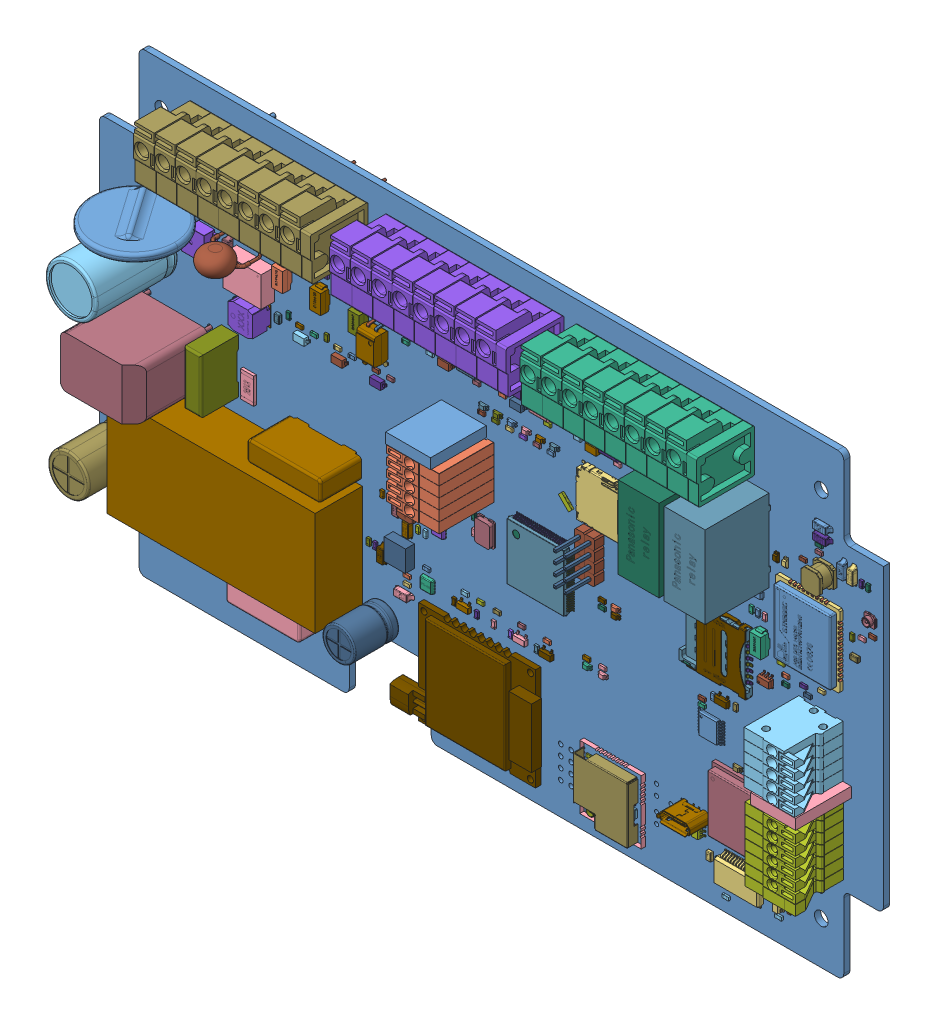
SolidWorks assembly Velvet_Controller_V1.2_2023, configuration Default. Lengths in mm. (continued)
Components (placement in the parent): (continued)
- Velvet_Controller_V1.2_2023(2)^Velvet_Controller_V1.2_2023-1: Velvet_Controller_V1.2_2023(2)^Velvet_Controller_V1.2_2023 [Default] at origin size (191.4 111.4 51.25) (virtual) (continued)
  - VD3gs^Velvet_Controller_V1.2_2023(2)_Velvet_Controller_V1.2_2023-1: VD3gs^Velvet_Controller_V1.2_2023(2)_Velvet_Controller_V1.2_2023 [Default] at origin size (2.79 5.49 2.29) (virtual) (continued)
    - DO-214AC(SMA)-2^VD3gs_Velvet_Controller_V1.2_2023(2)_Velvet_Controller_V1.2_2023-1: DO-214AC(SMA)-2^VD3gs_Velvet_Controller_V1.2_2023(2)_Velvet_Controller_V1.2_2023 [Default] at (162.275 62.25 0) x (0 1 0) z (1 0 0) size (5.49 2.29 2.79) (virtual)
  - VD2wf^Velvet_Controller_V1.2_2023(2)_Velvet_Controller_V1.2_2023-1: VD2wf^Velvet_Controller_V1.2_2023(2)_Velvet_Controller_V1.2_2023 [Default] at origin size (2.8 2.9 1.45) (virtual)
    - SOT23-6-2^VD2wf_Velvet_Controller_V1.2_2023(2)_Velvet_Controller_V1.2_2023-1: SOT23-6-2^VD2wf_Velvet_Controller_V1.2_2023(2)_Velvet_Controller_V1.2_2023 [Default] at (146.675 14.75 0) x (0 -1 0) z (0 0 1) size (2.9 2.8 1.45) (virtual)
  - VD2p^Velvet_Controller_V1.2_2023(2)_Velvet_Controller_V1.2_2023-1: VD2p^Velvet_Controller_V1.2_2023(2)_Velvet_Controller_V1.2_2023 [Default] at origin size (0.91 2.06 0.84) (virtual)
    - LED 0805^VD2p_Velvet_Controller_V1.2_2023(2)_Velvet_Controller_V1.2_2023-1: LED 0805^VD2p_Velvet_Controller_V1.2_2023(2)_Velvet_Controller_V1.2_2023 [Default] at (4.475 52.2282 0) x (-1 0 0) z (0 0 1) size (0.91 2.06 0.84) (virtual)
  - VD2mc^Velvet_Controller_V1.2_2023(2)_Velvet_Controller_V1.2_2023-1: VD2mc^Velvet_Controller_V1.2_2023(2)_Velvet_Controller_V1.2_2023 [Default] at origin size (2.06 0.91 0.84) (virtual)
    - LED 0805^VD2mc_Velvet_Controller_V1.2_2023(2)_Velvet_Controller_V1.2_2023-1: LED 0805^VD2mc_Velvet_Controller_V1.2_2023(2)_Velvet_Controller_V1.2_2023 [Default] at (108.6968 77.725 0) x (0 -1 0) z (0 0 1) size (0.91 2.06 0.84) (virtual)
  - VD2io^Velvet_Controller_V1.2_2023(2)_Velvet_Controller_V1.2_2023-1: VD2io^Velvet_Controller_V1.2_2023(2)_Velvet_Controller_V1.2_2023 [Default] at origin size (5.49 2.79 2.29) (virtual)
    - DO-214AC(SMA)-2^VD2io_Velvet_Controller_V1.2_2023(2)_Velvet_Controller_V1.2_2023-1: DO-214AC(SMA)-2^VD2io_Velvet_Controller_V1.2_2023(2)_Velvet_Controller_V1.2_2023 [Default] at (46.9 91.3 0) x (-1 0 0) z (0 1 0) size (5.49 2.29 2.79) (virtual)
  - VD2gs^Velvet_Controller_V1.2_2023(2)_Velvet_Controller_V1.2_2023-1: VD2gs^Velvet_Controller_V1.2_2023(2)_Velvet_Controller_V1.2_2023 [Default] at origin size (2.9 2.8 1.45) (virtual)
    - SOT23-6-2^VD2gs_Velvet_Controller_V1.2_2023(2)_Velvet_Controller_V1.2_2023-1: SOT23-6-2^VD2gs_Velvet_Controller_V1.2_2023(2)_Velvet_Controller_V1.2_2023 [Default] at (163.375 54.575 0) x (1 0 0) z (0 0 1) size (2.9 2.8 1.45) (virtual)
  - VD1wf^Velvet_Controller_V1.2_2023(2)_Velvet_Controller_V1.2_2023-1: VD1wf^Velvet_Controller_V1.2_2023(2)_Velvet_Controller_V1.2_2023 [Default] at origin size (2.06 0.91 0.84) (virtual)
    - LED 0805^VD1wf_Velvet_Controller_V1.2_2023(2)_Velvet_Controller_V1.2_2023-1: LED 0805^VD1wf_Velvet_Controller_V1.2_2023(2)_Velvet_Controller_V1.2_2023 [Default] at (155.3032 32.3 0) x (0 1 0) z (0 0 1) size (0.91 2.06 0.84) (virtual)
  - VD1p^Velvet_Controller_V1.2_2023(2)_Velvet_Controller_V1.2_2023-1: VD1p^Velvet_Controller_V1.2_2023(2)_Velvet_Controller_V1.2_2023 [Default] at origin size (1.6 3.7 1.15) (virtual)
    - SOD 123^VD1p_Velvet_Controller_V1.2_2023(2)_Velvet_Controller_V1.2_2023-1: SOD 123^VD1p_Velvet_Controller_V1.2_2023(2)_Velvet_Controller_V1.2_2023 [Default] at (16.5 80.4 0) x (0 -1 0) z (0 0 1) size (3.7 1.6 1.15) (virtual)
  - VD1mc^Velvet_Controller_V1.2_2023(2)_Velvet_Controller_V1.2_2023-1: VD1mc^Velvet_Controller_V1.2_2023(2)_Velvet_Controller_V1.2_2023 [Default] at origin size (2.06 0.91 0.84) (virtual)
    - LED 0805^VD1mc_Velvet_Controller_V1.2_2023(2)_Velvet_Controller_V1.2_2023-1: LED 0805^VD1mc_Velvet_Controller_V1.2_2023(2)_Velvet_Controller_V1.2_2023 [Default] at (112.1718 77.75 0) x (0 -1 0) z (0 0 1) size (0.91 2.06 0.84) (virtual)
  - VD1io^Velvet_Controller_V1.2_2023(2)_Velvet_Controller_V1.2_2023-1: VD1io^Velvet_Controller_V1.2_2023(2)_Velvet_Controller_V1.2_2023 [Default] at origin size (3.7 1.6 1.15) (virtual)
    - SOD 123^VD1io_Velvet_Controller_V1.2_2023(2)_Velvet_Controller_V1.2_2023-1: SOD 123^VD1io_Velvet_Controller_V1.2_2023(2)_Velvet_Controller_V1.2_2023 [Default] at (145.325 72.725 0) x (-1 0 0) z (0 0 1) size (3.7 1.6 1.15) (virtual)
  - VD1gs^Velvet_Controller_V1.2_2023(2)_Velvet_Controller_V1.2_2023-1: VD1gs^Velvet_Controller_V1.2_2023(2)_Velvet_Controller_V1.2_2023 [Default] at origin size (1.6 3.7 1.15) (virtual)
    - SOD 123^VD1gs_Velvet_Controller_V1.2_2023(2)_Velvet_Controller_V1.2_2023-1: SOD 123^VD1gs_Velvet_Controller_V1.2_2023(2)_Velvet_Controller_V1.2_2023 [Default] at (179.025 83.8 -1.5) x (0 -1 0) z (0 0 -1) size (3.7 1.6 1.15) (virtual)
  - U7io^Velvet_Controller_V1.2_2023(2)_Velvet_Controller_V1.2_2023-1: U7io^Velvet_Controller_V1.2_2023(2)_Velvet_Controller_V1.2_2023 [Default] at origin size (4.58 10 3.85) (virtual)
    - PC817_Gullwing^U7io_Velvet_Controller_V1.2_2023(2)_Velvet_Controller_V1.2_2023-1: PC817_Gullwing^U7io_Velvet_Controller_V1.2_2023(2)_Velvet_Controller_V1.2_2023 [Default] at (127.65 88.4 2.1) x (1 0 0) z (0 -1 0) size (4.58 3.85 10) (virtual)
      - PC817 Body^PC817_Gullwing_U7io_Velvet_Controller_V1.2_2023(2)_Velvet_Controller_V1.2_2023-1: PC817 Body^PC817_Gullwing_U7io_Velvet_Controller_V1.2_2023(2)_Velvet_Controller_V1.2_2023 [Default] at origin size (4.58 3.5 6.5) (virtual)
      - Gullwing Pin^PC817_Gullwing_U7io_Velvet_Controller_V1.2_2023(2)_Velvet_Controller_V1.2_2023-1: Gullwing Pin^PC817_Gullwing_U7io_Velvet_Controller_V1.2_2023(2)_Velvet_Controller_V1.2_2023 [Default] at (-13.5652 -2.1015 -0.2722) size (1.2 2.23 1.87) (virtual)
      - Gullwing Pin_MIR^PC817_Gullwing_U7io_Velvet_Controller_V1.2_2023(2)_Velvet_Controller_V1.2_2023-1: Gullwing Pin_MIR^PC817_Gullwing_U7io_Velvet_Controller_V1.2_2023(2)_Velvet_Controller_V1.2_2023 [Default] at (13.5652 -2.1015 -0.2722) x (-1 0 0) z (0 0 -1) size (1.2 2.23 1.87) (virtual)
      - Gullwing Pin_MIR1^PC817_Gullwing_U7io_Velvet_Controller_V1.2_2023(2)_Velvet_Controller_V1.2_2023-1: Gullwing Pin_MIR1^PC817_Gullwing_U7io_Velvet_Controller_V1.2_2023(2)_Velvet_Controller_V1.2_2023 [Default] at (-13.5652 -2.1015 0.2722) size (1.2 2.23 1.87) (virtual)
      - Gullwing Pin_MIR_MIR^PC817_Gullwing_U7io_Velvet_Controller_V1.2_2023(2)_Velvet_Controller_V1.2_2023-1: Gullwing Pin_MIR_MIR^PC817_Gullwing_U7io_Velvet_Controller_V1.2_2023(2)_Velvet_Controller_V1.2_2023 [Default] at (13.5652 -2.1015 0.2722) x (-1 0 0) z (0 0 -1) size (1.2 2.23 1.87) (virtual)
  - U6io^Velvet_Controller_V1.2_2023(2)_Velvet_Controller_V1.2_2023-1: U6io^Velvet_Controller_V1.2_2023(2)_Velvet_Controller_V1.2_2023 [Default] at origin size (4.58 10 3.85) (virtual)
    - PC817_Gullwing^U6io_Velvet_Controller_V1.2_2023(2)_Velvet_Controller_V1.2_2023-1: PC817_Gullwing^U6io_Velvet_Controller_V1.2_2023(2)_Velvet_Controller_V1.2_2023 [Default] at (110.65 88.4 2.1) x (1 0 0) z (0 -1 0) size (4.58 3.85 10) (virtual)
      - PC817 Body^PC817_Gullwing_U6io_Velvet_Controller_V1.2_2023(2)_Velvet_Controller_V1.2_2023-1: PC817 Body^PC817_Gullwing_U6io_Velvet_Controller_V1.2_2023(2)_Velvet_Controller_V1.2_2023 [Default] at origin size (4.58 3.5 6.5) (virtual)
      - Gullwing Pin^PC817_Gullwing_U6io_Velvet_Controller_V1.2_2023(2)_Velvet_Controller_V1.2_2023-1: Gullwing Pin^PC817_Gullwing_U6io_Velvet_Controller_V1.2_2023(2)_Velvet_Controller_V1.2_2023 [Default] at (-13.5652 -2.1015 -0.2722) size (1.2 2.23 1.87) (virtual)
      - Gullwing Pin_MIR^PC817_Gullwing_U6io_Velvet_Controller_V1.2_2023(2)_Velvet_Controller_V1.2_2023-1: Gullwing Pin_MIR^PC817_Gullwing_U6io_Velvet_Controller_V1.2_2023(2)_Velvet_Controller_V1.2_2023 [Default] at (13.5652 -2.1015 -0.2722) x (-1 0 0) z (0 0 -1) size (1.2 2.23 1.87) (virtual)
      - Gullwing Pin_MIR1^PC817_Gullwing_U6io_Velvet_Controller_V1.2_2023(2)_Velvet_Controller_V1.2_2023-1: Gullwing Pin_MIR1^PC817_Gullwing_U6io_Velvet_Controller_V1.2_2023(2)_Velvet_Controller_V1.2_2023 [Default] at (-13.5652 -2.1015 0.2722) size (1.2 2.23 1.87) (virtual)
      - Gullwing Pin_MIR_MIR^PC817_Gullwing_U6io_Velvet_Controller_V1.2_2023(2)_Velvet_Controller_V1.2_2023-1: Gullwing Pin_MIR_MIR^PC817_Gullwing_U6io_Velvet_Controller_V1.2_2023(2)_Velvet_Controller_V1.2_2023 [Default] at (13.5652 -2.1015 0.2722) x (-1 0 0) z (0 0 -1) size (1.2 2.23 1.87) (virtual)
  - U5io^Velvet_Controller_V1.2_2023(2)_Velvet_Controller_V1.2_2023-1: U5io^Velvet_Controller_V1.2_2023(2)_Velvet_Controller_V1.2_2023 [Default] at origin size (4.58 10 3.85) (virtual)
    - PC817_Gullwing^U5io_Velvet_Controller_V1.2_2023(2)_Velvet_Controller_V1.2_2023-1: PC817_Gullwing^U5io_Velvet_Controller_V1.2_2023(2)_Velvet_Controller_V1.2_2023 [Default] at (68.67 79.1 2.1) x (-1 0 0) z (0 1 0) size (4.58 3.85 10) (virtual)
      - PC817 Body^PC817_Gullwing_U5io_Velvet_Controller_V1.2_2023(2)_Velvet_Controller_V1.2_2023-1: PC817 Body^PC817_Gullwing_U5io_Velvet_Controller_V1.2_2023(2)_Velvet_Controller_V1.2_2023 [Default] at origin size (4.58 3.5 6.5) (virtual)
      - Gullwing Pin^PC817_Gullwing_U5io_Velvet_Controller_V1.2_2023(2)_Velvet_Controller_V1.2_2023-1: Gullwing Pin^PC817_Gullwing_U5io_Velvet_Controller_V1.2_2023(2)_Velvet_Controller_V1.2_2023 [Default] at (-13.5652 -2.1015 -0.2722) size (1.2 2.23 1.87) (virtual)
      - Gullwing Pin_MIR^PC817_Gullwing_U5io_Velvet_Controller_V1.2_2023(2)_Velvet_Controller_V1.2_2023-1: Gullwing Pin_MIR^PC817_Gullwing_U5io_Velvet_Controller_V1.2_2023(2)_Velvet_Controller_V1.2_2023 [Default] at (13.5652 -2.1015 -0.2722) x (-1 0 0) z (0 0 -1) size (1.2 2.23 1.87) (virtual)
      - Gullwing Pin_MIR1^PC817_Gullwing_U5io_Velvet_Controller_V1.2_2023(2)_Velvet_Controller_V1.2_2023-1: Gullwing Pin_MIR1^PC817_Gullwing_U5io_Velvet_Controller_V1.2_2023(2)_Velvet_Controller_V1.2_2023 [Default] at (-13.5652 -2.1015 0.2722) size (1.2 2.23 1.87) (virtual)
      - Gullwing Pin_MIR_MIR^PC817_Gullwing_U5io_Velvet_Controller_V1.2_2023(2)_Velvet_Controller_V1.2_2023-1: Gullwing Pin_MIR_MIR^PC817_Gullwing_U5io_Velvet_Controller_V1.2_2023(2)_Velvet_Controller_V1.2_2023 [Default] at (13.5652 -2.1015 0.2722) x (-1 0 0) z (0 0 -1) size (1.2 2.23 1.87) (virtual)
  - U4io^Velvet_Controller_V1.2_2023(2)_Velvet_Controller_V1.2_2023-1: U4io^Velvet_Controller_V1.2_2023(2)_Velvet_Controller_V1.2_2023 [Default] at origin size (4.58 10 3.85) (virtual)
    - PC817_Gullwing^U4io_Velvet_Controller_V1.2_2023(2)_Velvet_Controller_V1.2_2023-1: PC817_Gullwing^U4io_Velvet_Controller_V1.2_2023(2)_Velvet_Controller_V1.2_2023 [Default] at (93 88.5 2.1) x (1 0 0) z (0 -1 0) size (4.58 3.85 10) (virtual)
      - PC817 Body^PC817_Gullwing_U4io_Velvet_Controller_V1.2_2023(2)_Velvet_Controller_V1.2_2023-1: PC817 Body^PC817_Gullwing_U4io_Velvet_Controller_V1.2_2023(2)_Velvet_Controller_V1.2_2023 [Default] at origin size (4.58 3.5 6.5) (virtual)
      - Gullwing Pin^PC817_Gullwing_U4io_Velvet_Controller_V1.2_2023(2)_Velvet_Controller_V1.2_2023-1: Gullwing Pin^PC817_Gullwing_U4io_Velvet_Controller_V1.2_2023(2)_Velvet_Controller_V1.2_2023 [Default] at (-13.5652 -2.1015 -0.2722) size (1.2 2.23 1.87) (virtual)
      - Gullwing Pin_MIR^PC817_Gullwing_U4io_Velvet_Controller_V1.2_2023(2)_Velvet_Controller_V1.2_2023-1: Gullwing Pin_MIR^PC817_Gullwing_U4io_Velvet_Controller_V1.2_2023(2)_Velvet_Controller_V1.2_2023 [Default] at (13.5652 -2.1015 -0.2722) x (-1 0 0) z (0 0 -1) size (1.2 2.23 1.87) (virtual)
      - Gullwing Pin_MIR1^PC817_Gullwing_U4io_Velvet_Controller_V1.2_2023(2)_Velvet_Controller_V1.2_2023-1: Gullwing Pin_MIR1^PC817_Gullwing_U4io_Velvet_Controller_V1.2_2023(2)_Velvet_Controller_V1.2_2023 [Default] at (-13.5652 -2.1015 0.2722) size (1.2 2.23 1.87) (virtual)
      - Gullwing Pin_MIR_MIR^PC817_Gullwing_U4io_Velvet_Controller_V1.2_2023(2)_Velvet_Controller_V1.2_2023-1: Gullwing Pin_MIR_MIR^PC817_Gullwing_U4io_Velvet_Controller_V1.2_2023(2)_Velvet_Controller_V1.2_2023 [Default] at (13.5652 -2.1015 0.2722) x (-1 0 0) z (0 0 -1) size (1.2 2.23 1.87) (virtual)
  - U3io^Velvet_Controller_V1.2_2023(2)_Velvet_Controller_V1.2_2023-1: U3io^Velvet_Controller_V1.2_2023(2)_Velvet_Controller_V1.2_2023 [Default] at origin (virtual)
    - PC817_Gullwing.step-1: PC817_Gullwing.step [Default] at (59.3 79.1 2.1) x (-1 0 0) z (0 1 0) (suppressed, hidden)
  - U2io^Velvet_Controller_V1.2_2023(2)_Velvet_Controller_V1.2_2023-1: U2io^Velvet_Controller_V1.2_2023(2)_Velvet_Controller_V1.2_2023 [Default] at origin (virtual)
    - PC817_Gullwing.step-1: PC817_Gullwing.step [Default] at (75.925 88.4 2.1) x (1 0 0) z (0 -1 0) (suppressed, hidden)
  - U1io^Velvet_Controller_V1.2_2023(2)_Velvet_Controller_V1.2_2023-1: U1io^Velvet_Controller_V1.2_2023(2)_Velvet_Controller_V1.2_2023 [Default] at origin (virtual)
    - PC817_Gullwing.step-1: PC817_Gullwing.step [Default] at (50 79.1 2.1) x (-1 0 0) z (0 1 0) (suppressed, hidden)
  - RU1p^Velvet_Controller_V1.2_2023(2)_Velvet_Controller_V1.2_2023-1: RU1p^Velvet_Controller_V1.2_2023(2)_Velvet_Controller_V1.2_2023 [Default] at origin size (21 3.82 49.5) (virtual)
    - VARISTOR s20k275e2^RU1p_Velvet_Controller_V1.2_2023(2)_Velvet_Controller_V1.2_2023-1: VARISTOR s20k275e2^RU1p_Velvet_Controller_V1.2_2023(2)_Velvet_Controller_V1.2_2023 [Default] at (21.6 86.4 13) x (-1 0 0) z (0 1 0) size (21 49.5 3.82) (virtual)
  - R26io^Velvet_Controller_V1.2_2023(2)_Velvet_Controller_V1.2_2023-1: R26io^Velvet_Controller_V1.2_2023(2)_Velvet_Controller_V1.2_2023 [Default] at origin size (1.6 0.86 0.51) (virtual)
    - RES 0603^R26io_Velvet_Controller_V1.2_2023(2)_Velvet_Controller_V1.2_2023-1: RES 0603^R26io_Velvet_Controller_V1.2_2023(2)_Velvet_Controller_V1.2_2023 [Default] at (134.125 82.45 0) x (-1 0 0) z (0 1 0) size (1.6 0.51 0.86) (virtual)
  - R25io^Velvet_Controller_V1.2_2023(2)_Velvet_Controller_V1.2_2023-1: R25io^Velvet_Controller_V1.2_2023(2)_Velvet_Controller_V1.2_2023 [Default] at origin size (0.86 1.6 0.51) (virtual)
    - RES 0603^R25io_Velvet_Controller_V1.2_2023(2)_Velvet_Controller_V1.2_2023-1: RES 0603^R25io_Velvet_Controller_V1.2_2023(2)_Velvet_Controller_V1.2_2023 [Default] at (131 84.4 0) x (0 1 0) z (1 0 0) size (1.6 0.51 0.86) (virtual)
  - R24io^Velvet_Controller_V1.2_2023(2)_Velvet_Controller_V1.2_2023-1: R24io^Velvet_Controller_V1.2_2023(2)_Velvet_Controller_V1.2_2023 [Default] at origin size (1.6 0.86 0.51) (virtual)
    - RES 0603^R24io_Velvet_Controller_V1.2_2023(2)_Velvet_Controller_V1.2_2023-1: RES 0603^R24io_Velvet_Controller_V1.2_2023(2)_Velvet_Controller_V1.2_2023 [Default] at (126.725 81.825 0) x (-1 0 0) z (0 1 0) size (1.6 0.51 0.86) (virtual)
  - R23io^Velvet_Controller_V1.2_2023(2)_Velvet_Controller_V1.2_2023-1: R23io^Velvet_Controller_V1.2_2023(2)_Velvet_Controller_V1.2_2023 [Default] at origin size (1.6 0.86 0.51) (virtual)
    - RES 0603^R23io_Velvet_Controller_V1.2_2023(2)_Velvet_Controller_V1.2_2023-1: RES 0603^R23io_Velvet_Controller_V1.2_2023(2)_Velvet_Controller_V1.2_2023 [Default] at (117.05 82.475 0) x (-1 0 0) z (0 1 0) size (1.6 0.51 0.86) (virtual)
  - R22io^Velvet_Controller_V1.2_2023(2)_Velvet_Controller_V1.2_2023-1: R22io^Velvet_Controller_V1.2_2023(2)_Velvet_Controller_V1.2_2023 [Default] at origin size (0.86 1.6 0.51) (virtual)
    - RES 0603^R22io_Velvet_Controller_V1.2_2023(2)_Velvet_Controller_V1.2_2023-1: RES 0603^R22io_Velvet_Controller_V1.2_2023(2)_Velvet_Controller_V1.2_2023 [Default] at (114 84.4 0) x (0 1 0) z (1 0 0) size (1.6 0.51 0.86) (virtual)
  - R21io^Velvet_Controller_V1.2_2023(2)_Velvet_Controller_V1.2_2023-1: R21io^Velvet_Controller_V1.2_2023(2)_Velvet_Controller_V1.2_2023 [Default] at origin size (1.6 0.86 0.51) (virtual)
    - RES 0603^R21io_Velvet_Controller_V1.2_2023(2)_Velvet_Controller_V1.2_2023-1: RES 0603^R21io_Velvet_Controller_V1.2_2023(2)_Velvet_Controller_V1.2_2023 [Default] at (109.725 81.825 0) x (-1 0 0) z (0 1 0) size (1.6 0.51 0.86) (virtual)
  - R20lr^Velvet_Controller_V1.2_2023(2)_Velvet_Controller_V1.2_2023-1: R20lr^Velvet_Controller_V1.2_2023(2)_Velvet_Controller_V1.2_2023 [Default] at origin size (0.86 1.6 0.51) (virtual)
    - RES 0603^R20lr_Velvet_Controller_V1.2_2023(2)_Velvet_Controller_V1.2_2023-1: RES 0603^R20lr_Velvet_Controller_V1.2_2023(2)_Velvet_Controller_V1.2_2023 [Default] at (113.3 27.725 -1.5) x (0 1 0) z (-1 0 0) size (1.6 0.51 0.86) (virtual)
  - R20io^Velvet_Controller_V1.2_2023(2)_Velvet_Controller_V1.2_2023-1: R20io^Velvet_Controller_V1.2_2023(2)_Velvet_Controller_V1.2_2023 [Default] at origin size (0.86 1.6 0.51) (virtual)
    - RES 0603^R20io_Velvet_Controller_V1.2_2023(2)_Velvet_Controller_V1.2_2023-1: RES 0603^R20io_Velvet_Controller_V1.2_2023(2)_Velvet_Controller_V1.2_2023 [Default] at (65.08 73.1 0) x (0 -1 0) z (-1 0 0) size (1.6 0.51 0.86) (virtual)
  - R19lr^Velvet_Controller_V1.2_2023(2)_Velvet_Controller_V1.2_2023-1: R19lr^Velvet_Controller_V1.2_2023(2)_Velvet_Controller_V1.2_2023 [Default] at origin size (0.86 1.6 0.51) (virtual)
    - RES 0603^R19lr_Velvet_Controller_V1.2_2023(2)_Velvet_Controller_V1.2_2023-1: RES 0603^R19lr_Velvet_Controller_V1.2_2023(2)_Velvet_Controller_V1.2_2023 [Default] at (116.975 27.75 -1.5) x (0 1 0) z (-1 0 0) size (1.6 0.51 0.86) (virtual)
  - R19io^Velvet_Controller_V1.2_2023(2)_Velvet_Controller_V1.2_2023-1: R19io^Velvet_Controller_V1.2_2023(2)_Velvet_Controller_V1.2_2023 [Default] at origin size (1.6 0.86 0.51) (virtual)
    - RES 0603^R19io_Velvet_Controller_V1.2_2023(2)_Velvet_Controller_V1.2_2023-1: RES 0603^R19io_Velvet_Controller_V1.2_2023(2)_Velvet_Controller_V1.2_2023 [Default] at (67.78 72.2 0) x (-1 0 0) z (0 1 0) size (1.6 0.51 0.86) (virtual)
  - R18mc^Velvet_Controller_V1.2_2023(2)_Velvet_Controller_V1.2_2023-1: R18mc^Velvet_Controller_V1.2_2023(2)_Velvet_Controller_V1.2_2023 [Default] at origin size (0.86 1.6 0.51) (virtual)
    - RES 0603^R18mc_Velvet_Controller_V1.2_2023(2)_Velvet_Controller_V1.2_2023-1: RES 0603^R18mc_Velvet_Controller_V1.2_2023(2)_Velvet_Controller_V1.2_2023 [Default] at (155.55 44.85 0) x (0 1 0) z (1 0 0) size (1.6 0.51 0.86) (virtual)
  - R18lr^Velvet_Controller_V1.2_2023(2)_Velvet_Controller_V1.2_2023-1: R18lr^Velvet_Controller_V1.2_2023(2)_Velvet_Controller_V1.2_2023 [Default] at origin size (0.86 1.6 0.51) (virtual)
    - RES 0603^R18lr_Velvet_Controller_V1.2_2023(2)_Velvet_Controller_V1.2_2023-1: RES 0603^R18lr_Velvet_Controller_V1.2_2023(2)_Velvet_Controller_V1.2_2023 [Default] at (115.15 27.75 -1.5) x (0 1 0) z (-1 0 0) size (1.6 0.51 0.86) (virtual)
  - R18io^Velvet_Controller_V1.2_2023(2)_Velvet_Controller_V1.2_2023-1: R18io^Velvet_Controller_V1.2_2023(2)_Velvet_Controller_V1.2_2023 [Default] at origin size (0.86 1.6 0.51) (virtual)
    - RES 0603^R18io_Velvet_Controller_V1.2_2023(2)_Velvet_Controller_V1.2_2023-1: RES 0603^R18io_Velvet_Controller_V1.2_2023(2)_Velvet_Controller_V1.2_2023 [Default] at (65.08 86.4 0) x (0 -1 0) z (-1 0 0) size (1.6 0.51 0.86) (virtual)
  - R17mc^Velvet_Controller_V1.2_2023(2)_Velvet_Controller_V1.2_2023-1: R17mc^Velvet_Controller_V1.2_2023(2)_Velvet_Controller_V1.2_2023 [Default] at origin size (1.6 0.86 0.51) (virtual)
    - RES 0603^R17mc_Velvet_Controller_V1.2_2023(2)_Velvet_Controller_V1.2_2023-1: RES 0603^R17mc_Velvet_Controller_V1.2_2023(2)_Velvet_Controller_V1.2_2023 [Default] at (123.025 49.6 0) x (-1 0 0) z (0 1 0) size (1.6 0.51 0.86) (virtual)
  - R17lr^Velvet_Controller_V1.2_2023(2)_Velvet_Controller_V1.2_2023-1: R17lr^Velvet_Controller_V1.2_2023(2)_Velvet_Controller_V1.2_2023 [Default] at origin size (1.6 0.86 0.51) (virtual)
    - RES 0603^R17lr_Velvet_Controller_V1.2_2023(2)_Velvet_Controller_V1.2_2023-1: RES 0603^R17lr_Velvet_Controller_V1.2_2023(2)_Velvet_Controller_V1.2_2023 [Default] at (109.9 29.8 -1.5) x (-1 0 0) z (0 -1 0) size (1.6 0.51 0.86) (virtual)
  - R17io^Velvet_Controller_V1.2_2023(2)_Velvet_Controller_V1.2_2023-1: R17io^Velvet_Controller_V1.2_2023(2)_Velvet_Controller_V1.2_2023 [Default] at origin size (0.8 1.6 0.5) (virtual)
    - CAP 0603 (1608)^R17io_Velvet_Controller_V1.2_2023(2)_Velvet_Controller_V1.2_2023-1: CAP 0603 (1608)^R17io_Velvet_Controller_V1.2_2023(2)_Velvet_Controller_V1.2_2023 [Default] at (63 85.6 0) x (0 1 0) z (1 0 0) size (1.6 0.5 0.8) (virtual)
  - R16mc^Velvet_Controller_V1.2_2023(2)_Velvet_Controller_V1.2_2023-1: R16mc^Velvet_Controller_V1.2_2023(2)_Velvet_Controller_V1.2_2023 [Default] at origin size (1.6 0.86 0.51) (virtual)
    - RES 0603^R16mc_Velvet_Controller_V1.2_2023(2)_Velvet_Controller_V1.2_2023-1: RES 0603^R16mc_Velvet_Controller_V1.2_2023(2)_Velvet_Controller_V1.2_2023 [Default] at (123.025 51.15 0) x (-1 0 0) z (0 1 0) size (1.6 0.51 0.86) (virtual)
  - R16lr^Velvet_Controller_V1.2_2023(2)_Velvet_Controller_V1.2_2023-1: R16lr^Velvet_Controller_V1.2_2023(2)_Velvet_Controller_V1.2_2023 [Default] at origin size (1.6 0.86 0.51) (virtual)
    - RES 0603^R16lr_Velvet_Controller_V1.2_2023(2)_Velvet_Controller_V1.2_2023-1: RES 0603^R16lr_Velvet_Controller_V1.2_2023(2)_Velvet_Controller_V1.2_2023 [Default] at (106.45 27.95 -1.5) x (-1 0 0) z (0 -1 0) size (1.6 0.51 0.86) (virtual)
  - R16io^Velvet_Controller_V1.2_2023(2)_Velvet_Controller_V1.2_2023-1: R16io^Velvet_Controller_V1.2_2023(2)_Velvet_Controller_V1.2_2023 [Default] at origin size (1.6 0.86 0.51) (virtual)
    - RES 0603^R16io_Velvet_Controller_V1.2_2023(2)_Velvet_Controller_V1.2_2023-1: RES 0603^R16io_Velvet_Controller_V1.2_2023(2)_Velvet_Controller_V1.2_2023 [Default] at (98.75 82.45 0) x (-1 0 0) z (0 1 0) size (1.6 0.51 0.86) (virtual)
  - R15p^Velvet_Controller_V1.2_2023(2)_Velvet_Controller_V1.2_2023-1: R15p^Velvet_Controller_V1.2_2023(2)_Velvet_Controller_V1.2_2023 [Default] at origin size (0.86 1.6 0.51) (virtual)
    - RES 0603^R15p_Velvet_Controller_V1.2_2023(2)_Velvet_Controller_V1.2_2023-1: RES 0603^R15p_Velvet_Controller_V1.2_2023(2)_Velvet_Controller_V1.2_2023 [Default] at (84.225 29.5 -1.5) x (0 1 0) z (-1 0 0) size (1.6 0.51 0.86) (virtual)
  - R15mc^Velvet_Controller_V1.2_2023(2)_Velvet_Controller_V1.2_2023-1: R15mc^Velvet_Controller_V1.2_2023(2)_Velvet_Controller_V1.2_2023 [Default] at origin size (1.6 0.86 0.51) (virtual)
    - RES 0603^R15mc_Velvet_Controller_V1.2_2023(2)_Velvet_Controller_V1.2_2023-1: RES 0603^R15mc_Velvet_Controller_V1.2_2023(2)_Velvet_Controller_V1.2_2023 [Default] at (123.145 37 0) x (-1 0 0) z (0 1 0) size (1.6 0.51 0.86) (virtual)
  - R15lr^Velvet_Controller_V1.2_2023(2)_Velvet_Controller_V1.2_2023-1: R15lr^Velvet_Controller_V1.2_2023(2)_Velvet_Controller_V1.2_2023 [Default] at origin size (2.5 3.2 0.6) (virtual)
    - R_1210^R15lr_Velvet_Controller_V1.2_2023(2)_Velvet_Controller_V1.2_2023-1: R_1210^R15lr_Velvet_Controller_V1.2_2023(2)_Velvet_Controller_V1.2_2023 [Default] at (103.2 17.05 -1.5) x (0 1 0) z (0 0 -1) size (3.2 2.5 0.6) (virtual)
  - R15io^Velvet_Controller_V1.2_2023(2)_Velvet_Controller_V1.2_2023-1: R15io^Velvet_Controller_V1.2_2023(2)_Velvet_Controller_V1.2_2023 [Default] at origin size (1.6 0.86 0.51) (virtual)
    - RES 0603^R15io_Velvet_Controller_V1.2_2023(2)_Velvet_Controller_V1.2_2023-1: RES 0603^R15io_Velvet_Controller_V1.2_2023(2)_Velvet_Controller_V1.2_2023 [Default] at (157.325 70.825 0) x (1 0 0) z (0 -1 0) size (1.6 0.51 0.86) (virtual)
  - R15gs^Velvet_Controller_V1.2_2023(2)_Velvet_Controller_V1.2_2023-1: R15gs^Velvet_Controller_V1.2_2023(2)_Velvet_Controller_V1.2_2023 [Default] at origin size (1.6 0.86 0.51) (virtual)
    - RES 0603^R15gs_Velvet_Controller_V1.2_2023(2)_Velvet_Controller_V1.2_2023-1: RES 0603^R15gs_Velvet_Controller_V1.2_2023(2)_Velvet_Controller_V1.2_2023 [Default] at (171.625 70.725 -1.5) x (1 0 0) z (0 1 0) size (1.6 0.51 0.86) (virtual)
  - R14p^Velvet_Controller_V1.2_2023(2)_Velvet_Controller_V1.2_2023-1: R14p^Velvet_Controller_V1.2_2023(2)_Velvet_Controller_V1.2_2023 [Default] at origin size (0.86 1.6 0.51) (virtual)
    - RES 0603^R14p_Velvet_Controller_V1.2_2023(2)_Velvet_Controller_V1.2_2023-1: RES 0603^R14p_Velvet_Controller_V1.2_2023(2)_Velvet_Controller_V1.2_2023 [Default] at (78.725 29.525 -1.5) x (0 -1 0) z (1 0 0) size (1.6 0.51 0.86) (virtual)
  - R14mc^Velvet_Controller_V1.2_2023(2)_Velvet_Controller_V1.2_2023-1: R14mc^Velvet_Controller_V1.2_2023(2)_Velvet_Controller_V1.2_2023 [Default] at origin size (1.6 0.86 0.51) (virtual)
    - RES 0603^R14mc_Velvet_Controller_V1.2_2023(2)_Velvet_Controller_V1.2_2023-1: RES 0603^R14mc_Velvet_Controller_V1.2_2023(2)_Velvet_Controller_V1.2_2023 [Default] at (119.25 37 0) x (-1 0 0) z (0 1 0) size (1.6 0.51 0.86) (virtual)
  - R14lr^Velvet_Controller_V1.2_2023(2)_Velvet_Controller_V1.2_2023-1: R14lr^Velvet_Controller_V1.2_2023(2)_Velvet_Controller_V1.2_2023 [Default] at origin size (3.2 2.5 0.6) (virtual)
    - R_1210^R14lr_Velvet_Controller_V1.2_2023(2)_Velvet_Controller_V1.2_2023-1: R_1210^R14lr_Velvet_Controller_V1.2_2023(2)_Velvet_Controller_V1.2_2023 [Default] at (92.35 8.5 -1.5) x (1 0 0) z (0 0 -1) size (3.2 2.5 0.6) (virtual)
  - R14io^Velvet_Controller_V1.2_2023(2)_Velvet_Controller_V1.2_2023-1: R14io^Velvet_Controller_V1.2_2023(2)_Velvet_Controller_V1.2_2023 [Default] at origin size (0.86 1.6 0.51) (virtual)
    - RES 0603^R14io_Velvet_Controller_V1.2_2023(2)_Velvet_Controller_V1.2_2023-1: RES 0603^R14io_Velvet_Controller_V1.2_2023(2)_Velvet_Controller_V1.2_2023 [Default] at (96.3 84.5 0) x (0 1 0) z (1 0 0) size (1.6 0.51 0.86) (virtual)
  - R14gs^Velvet_Controller_V1.2_2023(2)_Velvet_Controller_V1.2_2023-1: R14gs^Velvet_Controller_V1.2_2023(2)_Velvet_Controller_V1.2_2023 [Default] at origin size (1.6 0.86 0.51) (virtual)
    - RES 0603^R14gs_Velvet_Controller_V1.2_2023(2)_Velvet_Controller_V1.2_2023-1: RES 0603^R14gs_Velvet_Controller_V1.2_2023(2)_Velvet_Controller_V1.2_2023 [Default] at (165.65 75.375 -1.5) x (1 0 0) z (0 1 0) size (1.6 0.51 0.86) (virtual)
  - R13p^Velvet_Controller_V1.2_2023(2)_Velvet_Controller_V1.2_2023-1: R13p^Velvet_Controller_V1.2_2023(2)_Velvet_Controller_V1.2_2023 [Default] at origin size (1.26 2.81 0.97) (virtual)
    - RES 0805^R13p_Velvet_Controller_V1.2_2023(2)_Velvet_Controller_V1.2_2023-1: RES 0805^R13p_Velvet_Controller_V1.2_2023(2)_Velvet_Controller_V1.2_2023 [Default] at (32.1 75.8 0) x (0 1 0) z (0 0 1) size (2.81 1.26 0.97) (virtual)
  - R13mc^Velvet_Controller_V1.2_2023(2)_Velvet_Controller_V1.2_2023-1: R13mc^Velvet_Controller_V1.2_2023(2)_Velvet_Controller_V1.2_2023 [Default] at origin size (1.6 0.86 0.51) (virtual)
    - RES 0603^R13mc_Velvet_Controller_V1.2_2023(2)_Velvet_Controller_V1.2_2023-1: RES 0603^R13mc_Velvet_Controller_V1.2_2023(2)_Velvet_Controller_V1.2_2023 [Default] at (77.325 56.825 0) x (1 0 0) z (0 -1 0) size (1.6 0.51 0.86) (virtual)
  - R13lr^Velvet_Controller_V1.2_2023(2)_Velvet_Controller_V1.2_2023-1: R13lr^Velvet_Controller_V1.2_2023(2)_Velvet_Controller_V1.2_2023 [Default] at origin size (2.5 3.2 0.6) (virtual)
    - R_1210^R13lr_Velvet_Controller_V1.2_2023(2)_Velvet_Controller_V1.2_2023-1: R_1210^R13lr_Velvet_Controller_V1.2_2023(2)_Velvet_Controller_V1.2_2023 [Default] at (83.7 16.95 -1.5) x (0 -1 0) z (0 0 -1) size (3.2 2.5 0.6) (virtual)
  - R13io^Velvet_Controller_V1.2_2023(2)_Velvet_Controller_V1.2_2023-1: R13io^Velvet_Controller_V1.2_2023(2)_Velvet_Controller_V1.2_2023 [Default] at origin size (0.86 1.6 0.51) (virtual)
    - RES 0603^R13io_Velvet_Controller_V1.2_2023(2)_Velvet_Controller_V1.2_2023-1: RES 0603^R13io_Velvet_Controller_V1.2_2023(2)_Velvet_Controller_V1.2_2023 [Default] at (55.71 73.1 0) x (0 -1 0) z (-1 0 0) size (1.6 0.51 0.86) (virtual)
  - R13gs^Velvet_Controller_V1.2_2023(2)_Velvet_Controller_V1.2_2023-1: R13gs^Velvet_Controller_V1.2_2023(2)_Velvet_Controller_V1.2_2023 [Default] at origin size (1.6 0.86 0.51) (virtual)
    - RES 0603^R13gs_Velvet_Controller_V1.2_2023(2)_Velvet_Controller_V1.2_2023-1: RES 0603^R13gs_Velvet_Controller_V1.2_2023(2)_Velvet_Controller_V1.2_2023 [Default] at (169.025 75.375 -1.5) x (1 0 0) z (0 1 0) size (1.6 0.51 0.86) (virtual)
  - R12p^Velvet_Controller_V1.2_2023(2)_Velvet_Controller_V1.2_2023-1: R12p^Velvet_Controller_V1.2_2023(2)_Velvet_Controller_V1.2_2023 [Default] at origin size (0.86 1.6 0.51) (virtual)
    - RES 0603^R12p_Velvet_Controller_V1.2_2023(2)_Velvet_Controller_V1.2_2023-1: RES 0603^R12p_Velvet_Controller_V1.2_2023(2)_Velvet_Controller_V1.2_2023 [Default] at (84.225 33.15 -1.5) x (0 1 0) z (-1 0 0) size (1.6 0.51 0.86) (virtual)
  - R12mc^Velvet_Controller_V1.2_2023(2)_Velvet_Controller_V1.2_2023-1: R12mc^Velvet_Controller_V1.2_2023(2)_Velvet_Controller_V1.2_2023 [Default] at origin size (1.6 0.86 0.51) (virtual)
    - RES 0603^R12mc_Velvet_Controller_V1.2_2023(2)_Velvet_Controller_V1.2_2023-1: RES 0603^R12mc_Velvet_Controller_V1.2_2023(2)_Velvet_Controller_V1.2_2023 [Default] at (77.325 55.025 0) x (1 0 0) z (0 -1 0) size (1.6 0.51 0.86) (virtual)
  - R12lr^Velvet_Controller_V1.2_2023(2)_Velvet_Controller_V1.2_2023-1: R12lr^Velvet_Controller_V1.2_2023(2)_Velvet_Controller_V1.2_2023 [Default] at origin size (3.2 2.5 0.6) (virtual)
    - R_1210^R12lr_Velvet_Controller_V1.2_2023(2)_Velvet_Controller_V1.2_2023-1: R_1210^R12lr_Velvet_Controller_V1.2_2023(2)_Velvet_Controller_V1.2_2023 [Default] at (92.35 26.6 -1.5) x (-1 0 0) z (0 0 -1) size (3.2 2.5 0.6) (virtual)
  - R12io^Velvet_Controller_V1.2_2023(2)_Velvet_Controller_V1.2_2023-1: R12io^Velvet_Controller_V1.2_2023(2)_Velvet_Controller_V1.2_2023 [Default] at origin size (1.6 0.86 0.51) (virtual)
    - RES 0603^R12io_Velvet_Controller_V1.2_2023(2)_Velvet_Controller_V1.2_2023-1: RES 0603^R12io_Velvet_Controller_V1.2_2023(2)_Velvet_Controller_V1.2_2023 [Default] at (58.41 72.2 0) x (-1 0 0) z (0 1 0) size (1.6 0.51 0.86) (virtual)
  - R12gs^Velvet_Controller_V1.2_2023(2)_Velvet_Controller_V1.2_2023-1: R12gs^Velvet_Controller_V1.2_2023(2)_Velvet_Controller_V1.2_2023 [Default] at origin size (0.86 1.6 0.51) (virtual)
    - RES 0603^R12gs_Velvet_Controller_V1.2_2023(2)_Velvet_Controller_V1.2_2023-1: RES 0603^R12gs_Velvet_Controller_V1.2_2023(2)_Velvet_Controller_V1.2_2023 [Default] at (162.65 67.5 0) x (0 1 0) z (1 0 0) size (1.6 0.51 0.86) (virtual)
  - R11p^Velvet_Controller_V1.2_2023(2)_Velvet_Controller_V1.2_2023-1: R11p^Velvet_Controller_V1.2_2023(2)_Velvet_Controller_V1.2_2023 [Default] at origin size (1.6 0.86 0.51) (virtual)
    - RES 0603^R11p_Velvet_Controller_V1.2_2023(2)_Velvet_Controller_V1.2_2023-1: RES 0603^R11p_Velvet_Controller_V1.2_2023(2)_Velvet_Controller_V1.2_2023 [Default] at (81.55 35.875 -1.5) x (1 0 0) z (0 1 0) size (1.6 0.51 0.86) (virtual)
  - R11mc^Velvet_Controller_V1.2_2023(2)_Velvet_Controller_V1.2_2023-1: R11mc^Velvet_Controller_V1.2_2023(2)_Velvet_Controller_V1.2_2023 [Default] at origin size (1.6 0.86 0.51) (virtual)
    - RES 0603^R11mc_Velvet_Controller_V1.2_2023(2)_Velvet_Controller_V1.2_2023-1: RES 0603^R11mc_Velvet_Controller_V1.2_2023(2)_Velvet_Controller_V1.2_2023 [Default] at (77.325 53.35 0) x (1 0 0) z (0 -1 0) size (1.6 0.51 0.86) (virtual)
  - R11lr^Velvet_Controller_V1.2_2023(2)_Velvet_Controller_V1.2_2023-1: R11lr^Velvet_Controller_V1.2_2023(2)_Velvet_Controller_V1.2_2023 [Default] at origin size (1.6 0.86 0.51) (virtual)
    - RES 0603^R11lr_Velvet_Controller_V1.2_2023(2)_Velvet_Controller_V1.2_2023-1: RES 0603^R11lr_Velvet_Controller_V1.2_2023(2)_Velvet_Controller_V1.2_2023 [Default] at (93.3 35.9 0) x (-1 0 0) z (0 1 0) size (1.6 0.51 0.86) (virtual)
  - R11io^Velvet_Controller_V1.2_2023(2)_Velvet_Controller_V1.2_2023-1: R11io^Velvet_Controller_V1.2_2023(2)_Velvet_Controller_V1.2_2023 [Default] at origin size (0.86 1.6 0.51) (virtual)
    - RES 0603^R11io_Velvet_Controller_V1.2_2023(2)_Velvet_Controller_V1.2_2023-1: RES 0603^R11io_Velvet_Controller_V1.2_2023(2)_Velvet_Controller_V1.2_2023 [Default] at (55.71 86.4 0) x (0 -1 0) z (-1 0 0) size (1.6 0.51 0.86) (virtual)
  - R11gs^Velvet_Controller_V1.2_2023(2)_Velvet_Controller_V1.2_2023-1: R11gs^Velvet_Controller_V1.2_2023(2)_Velvet_Controller_V1.2_2023 [Default] at origin size (0.86 1.6 0.51) (virtual)
    - RES 0603^R11gs_Velvet_Controller_V1.2_2023(2)_Velvet_Controller_V1.2_2023-1: RES 0603^R11gs_Velvet_Controller_V1.2_2023(2)_Velvet_Controller_V1.2_2023 [Default] at (165.575 81.625 -1.5) x (0 -1 0) z (1 0 0) size (1.6 0.51 0.86) (virtual)
  - R10p^Velvet_Controller_V1.2_2023(2)_Velvet_Controller_V1.2_2023-1: R10p^Velvet_Controller_V1.2_2023(2)_Velvet_Controller_V1.2_2023 [Default] at origin size (0.86 1.6 0.51) (virtual)
    - RES 0603^R10p_Velvet_Controller_V1.2_2023(2)_Velvet_Controller_V1.2_2023-1: RES 0603^R10p_Velvet_Controller_V1.2_2023(2)_Velvet_Controller_V1.2_2023 [Default] at (86.8247 41.8694 -1.5) x (0 1 0) z (-1 0 0) size (1.6 0.51 0.86) (virtual)
  - R10mc^Velvet_Controller_V1.2_2023(2)_Velvet_Controller_V1.2_2023-1: R10mc^Velvet_Controller_V1.2_2023(2)_Velvet_Controller_V1.2_2023 [Default] at origin size (1.6 0.86 0.51) (virtual)
    - RES 0603^R10mc_Velvet_Controller_V1.2_2023(2)_Velvet_Controller_V1.2_2023-1: RES 0603^R10mc_Velvet_Controller_V1.2_2023(2)_Velvet_Controller_V1.2_2023 [Default] at (93.55 76.125 0) x (1 0 0) z (0 -1 0) size (1.6 0.51 0.86) (virtual)
  - R10lr^Velvet_Controller_V1.2_2023(2)_Velvet_Controller_V1.2_2023-1: R10lr^Velvet_Controller_V1.2_2023(2)_Velvet_Controller_V1.2_2023 [Default] at origin size (1.6 0.86 0.51) (virtual)
    - RES 0603^R10lr_Velvet_Controller_V1.2_2023(2)_Velvet_Controller_V1.2_2023-1: RES 0603^R10lr_Velvet_Controller_V1.2_2023(2)_Velvet_Controller_V1.2_2023 [Default] at (97.4 35.9 0) x (-1 0 0) z (0 1 0) size (1.6 0.51 0.86) (virtual)
  - R10io^Velvet_Controller_V1.2_2023(2)_Velvet_Controller_V1.2_2023-1: R10io^Velvet_Controller_V1.2_2023(2)_Velvet_Controller_V1.2_2023 [Default] at origin size (1.6 0.86 0.51) (virtual)
    - RES 0603^R10io_Velvet_Controller_V1.2_2023(2)_Velvet_Controller_V1.2_2023-1: RES 0603^R10io_Velvet_Controller_V1.2_2023(2)_Velvet_Controller_V1.2_2023 [Default] at (92.36 81.825 0) x (-1 0 0) z (0 1 0) size (1.6 0.51 0.86) (virtual)
  - R10gs^Velvet_Controller_V1.2_2023(2)_Velvet_Controller_V1.2_2023-1: R10gs^Velvet_Controller_V1.2_2023(2)_Velvet_Controller_V1.2_2023 [Default] at origin size (0.86 1.6 0.51) (virtual)
    - RES 0603^R10gs_Velvet_Controller_V1.2_2023(2)_Velvet_Controller_V1.2_2023-1: RES 0603^R10gs_Velvet_Controller_V1.2_2023(2)_Velvet_Controller_V1.2_2023 [Default] at (167.825 81.6 -1.5) x (0 -1 0) z (1 0 0) size (1.6 0.51 0.86) (virtual)
  - R9p^Velvet_Controller_V1.2_2023(2)_Velvet_Controller_V1.2_2023-1: R9p^Velvet_Controller_V1.2_2023(2)_Velvet_Controller_V1.2_2023 [Default] at origin size (0.86 1.6 0.51) (virtual)
    - RES 0603^R9p_Velvet_Controller_V1.2_2023(2)_Velvet_Controller_V1.2_2023-1: RES 0603^R9p_Velvet_Controller_V1.2_2023(2)_Velvet_Controller_V1.2_2023 [Default] at (168.4 91 -1.5) x (0 -1 0) z (1 0 0) size (1.6 0.51 0.86) (virtual)
  - R9mc^Velvet_Controller_V1.2_2023(2)_Velvet_Controller_V1.2_2023-1: R9mc^Velvet_Controller_V1.2_2023(2)_Velvet_Controller_V1.2_2023 [Default] at origin size (1.6 0.86 0.51) (virtual)
    - RES 0603^R9mc_Velvet_Controller_V1.2_2023(2)_Velvet_Controller_V1.2_2023-1: RES 0603^R9mc_Velvet_Controller_V1.2_2023(2)_Velvet_Controller_V1.2_2023 [Default] at (96.95 76.125 0) x (1 0 0) z (0 -1 0) size (1.6 0.51 0.86) (virtual)
  - R9lr^Velvet_Controller_V1.2_2023(2)_Velvet_Controller_V1.2_2023-1: R9lr^Velvet_Controller_V1.2_2023(2)_Velvet_Controller_V1.2_2023 [Default] at origin size (0.86 1.6 0.51) (virtual)
    - RES 0603^R9lr_Velvet_Controller_V1.2_2023(2)_Velvet_Controller_V1.2_2023-1: RES 0603^R9lr_Velvet_Controller_V1.2_2023(2)_Velvet_Controller_V1.2_2023 [Default] at (92.4 32.9 0) x (0 -1 0) z (-1 0 0) size (1.6 0.51 0.86) (virtual)
  - R9io^Velvet_Controller_V1.2_2023(2)_Velvet_Controller_V1.2_2023-1: R9io^Velvet_Controller_V1.2_2023(2)_Velvet_Controller_V1.2_2023 [Default] at origin size (0.8 1.6 0.5) (virtual)
    - CAP 0603 (1608)^R9io_Velvet_Controller_V1.2_2023(2)_Velvet_Controller_V1.2_2023-1: CAP 0603 (1608)^R9io_Velvet_Controller_V1.2_2023(2)_Velvet_Controller_V1.2_2023 [Default] at (54 85.6 0) x (0 1 0) z (1 0 0) size (1.6 0.5 0.8) (virtual)
  - R9gs^Velvet_Controller_V1.2_2023(2)_Velvet_Controller_V1.2_2023-1: R9gs^Velvet_Controller_V1.2_2023(2)_Velvet_Controller_V1.2_2023 [Default] at origin size (0.86 1.6 0.51) (virtual)
    - RES 0603^R9gs_Velvet_Controller_V1.2_2023(2)_Velvet_Controller_V1.2_2023-1: RES 0603^R9gs_Velvet_Controller_V1.2_2023(2)_Velvet_Controller_V1.2_2023 [Default] at (161 67.5 0) x (0 -1 0) z (-1 0 0) size (1.6 0.51 0.86) (virtual)
  - R8p^Velvet_Controller_V1.2_2023(2)_Velvet_Controller_V1.2_2023-1: R8p^Velvet_Controller_V1.2_2023(2)_Velvet_Controller_V1.2_2023 [Default] at origin size (0.86 1.6 0.51) (virtual)
    - RES 0603^R8p_Velvet_Controller_V1.2_2023(2)_Velvet_Controller_V1.2_2023-1: RES 0603^R8p_Velvet_Controller_V1.2_2023(2)_Velvet_Controller_V1.2_2023 [Default] at (81.4247 41.8694 -1.5) x (0 1 0) z (-1 0 0) size (1.6 0.51 0.86) (virtual)
  - R8mc^Velvet_Controller_V1.2_2023(2)_Velvet_Controller_V1.2_2023-1: R8mc^Velvet_Controller_V1.2_2023(2)_Velvet_Controller_V1.2_2023 [Default] at origin size (1.6 0.86 0.51) (virtual)
    - RES 0603^R8mc_Velvet_Controller_V1.2_2023(2)_Velvet_Controller_V1.2_2023-1: RES 0603^R8mc_Velvet_Controller_V1.2_2023(2)_Velvet_Controller_V1.2_2023 [Default] at (100.35 76.125 0) x (1 0 0) z (0 -1 0) size (1.6 0.51 0.86) (virtual)
  - R8lr^Velvet_Controller_V1.2_2023(2)_Velvet_Controller_V1.2_2023-1: R8lr^Velvet_Controller_V1.2_2023(2)_Velvet_Controller_V1.2_2023 [Default] at origin size (0.86 1.6 0.51) (virtual)
    - RES 0603^R8lr_Velvet_Controller_V1.2_2023(2)_Velvet_Controller_V1.2_2023-1: RES 0603^R8lr_Velvet_Controller_V1.2_2023(2)_Velvet_Controller_V1.2_2023 [Default] at (96.5 32.9 0) x (0 -1 0) z (-1 0 0) size (1.6 0.51 0.86) (virtual)
  - R8io^Velvet_Controller_V1.2_2023(2)_Velvet_Controller_V1.2_2023-1: R8io^Velvet_Controller_V1.2_2023(2)_Velvet_Controller_V1.2_2023 [Default] at origin size (1.6 0.86 0.51) (virtual)
    - RES 0603^R8io_Velvet_Controller_V1.2_2023(2)_Velvet_Controller_V1.2_2023-1: RES 0603^R8io_Velvet_Controller_V1.2_2023(2)_Velvet_Controller_V1.2_2023 [Default] at (81.05 82.4 0) x (-1 0 0) z (0 1 0) size (1.6 0.51 0.86) (virtual)
  - R8gs^Velvet_Controller_V1.2_2023(2)_Velvet_Controller_V1.2_2023-1: R8gs^Velvet_Controller_V1.2_2023(2)_Velvet_Controller_V1.2_2023 [Default] at origin size (0.86 1.6 0.51) (virtual)
    - RES 0603^R8gs_Velvet_Controller_V1.2_2023(2)_Velvet_Controller_V1.2_2023-1: RES 0603^R8gs_Velvet_Controller_V1.2_2023(2)_Velvet_Controller_V1.2_2023 [Default] at (159.425 67.525 0) x (0 -1 0) z (-1 0 0) size (1.6 0.51 0.86) (virtual)
  - R7p^Velvet_Controller_V1.2_2023(2)_Velvet_Controller_V1.2_2023-1: R7p^Velvet_Controller_V1.2_2023(2)_Velvet_Controller_V1.2_2023 [Default] at origin size (0.86 1.6 0.51) (virtual)
    - RES 0603^R7p_Velvet_Controller_V1.2_2023(2)_Velvet_Controller_V1.2_2023-1: RES 0603^R7p_Velvet_Controller_V1.2_2023(2)_Velvet_Controller_V1.2_2023 [Default] at (173.4 91 -1.5) x (0 -1 0) z (1 0 0) size (1.6 0.51 0.86) (virtual)
  - R7mc^Velvet_Controller_V1.2_2023(2)_Velvet_Controller_V1.2_2023-1: R7mc^Velvet_Controller_V1.2_2023(2)_Velvet_Controller_V1.2_2023 [Default] at origin size (1.6 0.86 0.51) (virtual)
    - RES 0603^R7mc_Velvet_Controller_V1.2_2023(2)_Velvet_Controller_V1.2_2023-1: RES 0603^R7mc_Velvet_Controller_V1.2_2023(2)_Velvet_Controller_V1.2_2023 [Default] at (103.75 76.125 0) x (1 0 0) z (0 -1 0) size (1.6 0.51 0.86) (virtual)
  - R7lr^Velvet_Controller_V1.2_2023(2)_Velvet_Controller_V1.2_2023-1: R7lr^Velvet_Controller_V1.2_2023(2)_Velvet_Controller_V1.2_2023 [Default] at origin size (0.86 1.6 0.51) (virtual)
    - RES 0603^R7lr_Velvet_Controller_V1.2_2023(2)_Velvet_Controller_V1.2_2023-1: RES 0603^R7lr_Velvet_Controller_V1.2_2023(2)_Velvet_Controller_V1.2_2023 [Default] at (132.18 19.001 -1.5) x (0 1 0) z (-1 0 0) size (1.6 0.51 0.86) (virtual)
  - R7io^Velvet_Controller_V1.2_2023(2)_Velvet_Controller_V1.2_2023-1: R7io^Velvet_Controller_V1.2_2023(2)_Velvet_Controller_V1.2_2023 [Default] at origin size (1.6 0.86 0.51) (virtual)
    - RES 0603^R7io_Velvet_Controller_V1.2_2023(2)_Velvet_Controller_V1.2_2023-1: RES 0603^R7io_Velvet_Controller_V1.2_2023(2)_Velvet_Controller_V1.2_2023 [Default] at (145.95 70.8 0) x (1 0 0) z (0 -1 0) size (1.6 0.51 0.86) (virtual)
  - R7gs^Velvet_Controller_V1.2_2023(2)_Velvet_Controller_V1.2_2023-1: R7gs^Velvet_Controller_V1.2_2023(2)_Velvet_Controller_V1.2_2023 [Default] at origin size (1.6 0.86 0.51) (virtual)
    - RES 0603^R7gs_Velvet_Controller_V1.2_2023(2)_Velvet_Controller_V1.2_2023-1: RES 0603^R7gs_Velvet_Controller_V1.2_2023(2)_Velvet_Controller_V1.2_2023 [Default] at (188.95 76.425 0) x (-1 0 0) z (0 1 0) size (1.6 0.51 0.86) (virtual)
  - R6p^Velvet_Controller_V1.2_2023(2)_Velvet_Controller_V1.2_2023-1: R6p^Velvet_Controller_V1.2_2023(2)_Velvet_Controller_V1.2_2023 [Default] at origin size (0.86 1.6 0.51) (virtual)
    - RES 0603^R6p_Velvet_Controller_V1.2_2023(2)_Velvet_Controller_V1.2_2023-1: RES 0603^R6p_Velvet_Controller_V1.2_2023(2)_Velvet_Controller_V1.2_2023 [Default] at (86.8247 45.4693 -1.5) x (0 -1 0) z (1 0 0) size (1.6 0.51 0.86) (virtual)
  - R6mc^Velvet_Controller_V1.2_2023(2)_Velvet_Controller_V1.2_2023-1: R6mc^Velvet_Controller_V1.2_2023(2)_Velvet_Controller_V1.2_2023 [Default] at origin size (1.6 0.86 0.51) (virtual)
    - RES 0603^R6mc_Velvet_Controller_V1.2_2023(2)_Velvet_Controller_V1.2_2023-1: RES 0603^R6mc_Velvet_Controller_V1.2_2023(2)_Velvet_Controller_V1.2_2023 [Default] at (107.15 76.125 0) x (1 0 0) z (0 -1 0) size (1.6 0.51 0.86) (virtual)
